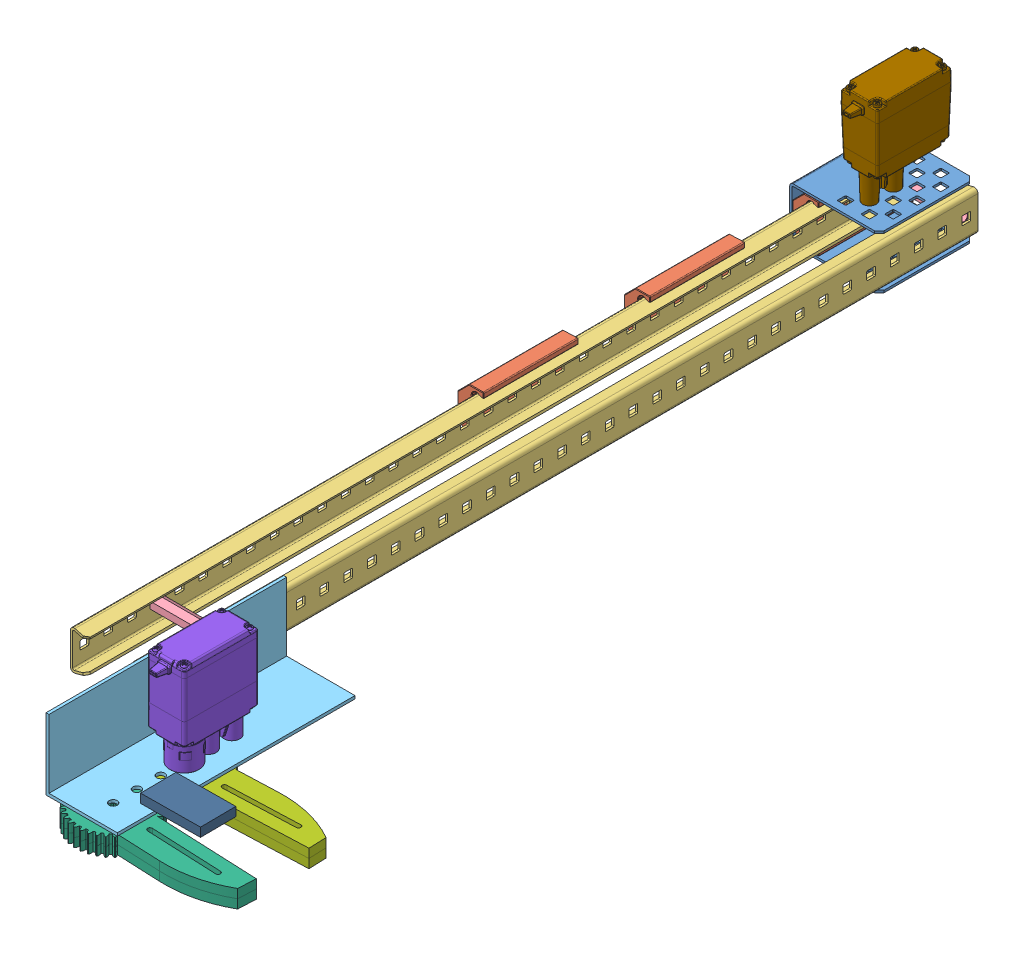
SolidWorks assembly ClawAssy-NoMates, configuration Default. Lengths in mm.
Overall size (145.25 95.98 508.56).
16 component instances, 10 part files, 0 mates.
Components (placement in the parent):
- 276-1926-002 Rev1-1: 276-1926-002 Rev1 [Default] at (-137.3124 83.7946 -100.4316) x (0 1 0) z (1 0 0) size (28.68 50.8 47.88)
- 276-1926-004 Rev1-1: 276-1926-004 Rev1 [Default] at (-127.9844 83.7946 -100.4316) x (0 -1 0) z (0 0 1) size (25.39 14.24 50.81)
- 276-1926-004 Rev1-2: 276-1926-004 Rev1 [Default] at (-129.1844 83.7946 -11.5316) x (0 -1 0) z (0 0 1) size (25.39 14.24 50.81)
- 276-1926-004 Rev1-3: 276-1926-004 Rev1 [Default] at (-129.1844 83.7946 77.3684) x (0 -1 0) z (0 0 1) size (25.39 14.24 50.81)
- 276-1926-005 Rev1-1: 276-1926-005 Rev1 [Default] at (-87.4844 83.7946 166.2684) x (0 1 0) z (-1 0 0) size (20.84 444.5 8.8)
- 276-1926-005 Rev1-2: 276-1926-005 Rev1 [Default] at (-127.9844 83.7946 166.2684) x (0 -1 0) z (1 0 0) size (20.84 444.5 8.8)
- BEAM-1500-1: BEAM-1500 [Default] at (-107.7344 83.7946 -119.4816) x (0 1 0) z (0 0 1) size (7.34 38.98 7.34)
- BEAM-1500-2: BEAM-1500 [Default] at (-107.7344 83.7946 274.2184) x (0 1 0) z (0 0 1) size (7.34 38.98 7.34)
- Claw-Bracket-1: Claw-Bracket [Default] at (-87.4844 62.8839 245.1926) size (38.1 38.1 127)
- CLAW_L-1: CLAW_L [Default] at (-64.3069 58.1214 359.4926) x (0.044064 0 -0.999029) z (0 1 0) size (40.21 91.53 4.76)
- CLAW_L-2: CLAW_L [Default] at (-64.3069 53.3589 359.4926) x (0.044064 0 -0.999029) z (0 1 0) size (40.21 91.53 4.76)
- CLAW_R-1: CLAW_R [Default] at (-64.3069 58.1214 321.3926) x (-0.03894 0 -0.999242) z (0 1 0) size (40.15 91.5 4.76)
- CLAW_R-2: CLAW_R [Default] at (-64.3069 53.3589 321.3926) x (-0.03894 0 -0.999242) z (0 1 0) size (40.15 91.5 4.76)
- VEX-MOTOR-1: VEX-MOTOR [Default] at (-64.3069 92.5714 311.4926) x (0 0 1) z (0 1 0) size (46.84 20 53.77)
- VEX-2WIRE-MOTOR-1: VEX-2WIRE-MOTOR [Default] at (-107.3658 141.3329 -102.0018) x (0 0 -1) z (0 1 0) size (46.4 20 51.81)
- magmount-1: magmount [Default] at (-25.0031 64.4714 352.1194) x (-0.008727 0 -0.999962) z (0 1 0) size (19.05 31.75 4.76)
